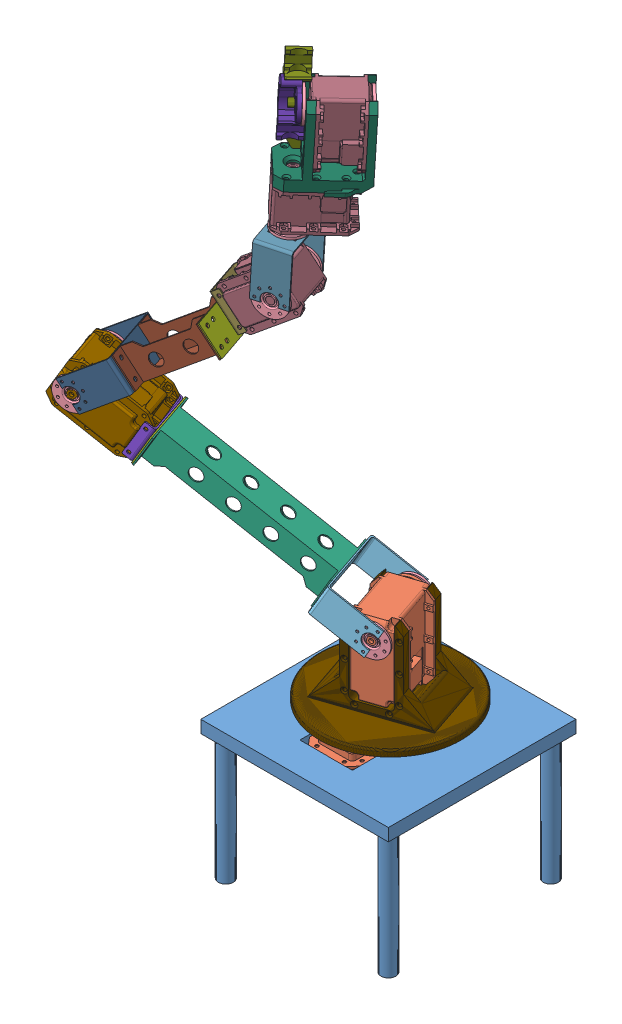
SolidWorks assembly Crust crawler, configuration Default. Lengths in mm.
Overall size (286.73 536.38 160.83).
31 component instances, 18 part files, 69 mates.
Components (placement in the parent):
- Base-1: Base [Default] at (55.1013 113.759 122.0745) size (150 110 150)
- MX-106T-1: MX-106T [Default] at (56.0013 106.759 121.3245) x (1 0 0) z (0 1 0) size (40.2 65.92 55.3)
- Base-disc-1: Base-disc [Default] at (56.0013 136.559 121.3245) x (-0.957483 0 0.288489) z (-0.288489 0 -0.957483) size (110 1 110)
- MX-106T-2: MX-106T [Default] at (55.9531 193.559 121.3159) x (-0.946958 0 0.321357) z (-0.321357 0 -0.946958) size (40.2 65.92 55.3)
- Servo-Disc-2: Servo-Disc [Default] at (46.698 193.559 94.0435) x (-0.321357 0 -0.946958) z (0.946958 0 -0.321357) size (2 25 25)
- Servo-Disc-3: Servo-Disc [Default] at (63.1836 193.559 142.6225) x (0.321357 0 0.946958) z (-0.826712 0.487687 0.28055) size (2 25 25)
- Servo-disc-link_MX-106T-2: Servo-disc-link_MX-106T [Default] at (15.7767 201.1783 125.1291) x (0.321357 0 0.946958) z (-0.826712 0.487687 0.28055) size (57.3 25 41)
- Link-1-1: Link-1 [Default] at (-24.8512 254.9473 145.4109) x (-0.321357 0 -0.946958) z (-0.826712 0.487687 0.28055) size (45 25 130)
- Link-plate-1: Link-plate [Default] at (-84.3602 275.7342 165.6057) x (-0.321357 0 -0.946958) z (-0.826712 0.487687 0.28055) size (45 25 1)
- Servo-link-link_MX-64T-1: Servo-link-link_MX-64T [Default] at (-93.9736 263.3704 164.1161) x (-0.321357 0 -0.946958) z (0.826712 -0.487687 -0.28055) size (36 30 8)
- MX-64T-1: MX-64T [Default] at (-126.7705 300.7525 179.998) x (-0.461819 -0.873019 0.156721) z (-0.321357 0 -0.946958) size (40.2 62.1 50)
- Servo-Disc-4: Servo-Disc [Default] at (-135.1258 300.7525 155.3771) x (-0.321357 0 -0.946958) z (0.934807 -0.159687 -0.317233) size (2 25 25)
- Servo-Disc-5: Servo-Disc [Default] at (-120.3434 300.7525 198.9372) x (0.321357 0 0.946958) z (0.288069 0.952607 -0.097758) size (2 25 25)
- Servo-disc-link_MX-64T-1: Servo-disc-link_MX-64T [Default] at (-90.5023 312.8501 168.2181) x (-0.321357 0 -0.946958) z (0.767934 0.585117 -0.260604) size (52 25 41)
- Link-2-1: Link-2 [Default] at (-65.5173 332.7441 156.0432) x (-0.321357 0 -0.946958) z (0.767934 0.585117 -0.260604) size (45 25 67)
- Link-plate-2: Link-plate [Default] at (-46.7175 362.4824 149.6634) x (0.321357 0 0.946958) z (0.767934 0.585117 -0.260604) size (45 25 1)
- Servo-link-link_MX-28T-1: Servo-link-link_MX-28T [Default] at (-42.8849 355.2506 138.9643) x (0.321357 0 0.946958) z (-0.767934 -0.585117 0.260604) size (32 30 8)
- MX-28T-1: MX-28T [Default] at (-22.3058 390.9491 125.1165) x (0.554082 -0.810949 -0.188031) z (0.321357 0 0.946958) size (35.6 50.71 41.85)
- Servo-Disc-6: Servo-Disc [Default] at (-15.6858 390.9491 144.6239) x (0.321357 0 0.946958) z (0.945652 -0.052502 -0.320914) size (2 25 25)
- Servo-Disc-8: Servo-Disc [Default] at (-27.8492 390.9491 108.7815) x (-0.321357 0 -0.946958) z (0.909105 -0.279908 -0.308511) size (2 25 25)
- Servo-disc-link_MX-28T-2: Servo-disc-link_MX-28T [Default] at (-31.5141 429.553 130.6175) x (0.321357 0 0.946958) z (0.049717 0.998621 -0.016872) size (43.85 25 41)
- Servo-Disc-10: Servo-Disc [Default] at (-19.754 431.3933 126.0194) x (-0.049717 -0.998621 0.016872) z (0.75968 -0.048777 -0.648465) size (2 25 25)
- Servo-Disc-11: Servo-Disc [Default] at (-17.8722 469.1911 125.3808) x (0.049717 0.998621 -0.016872) z (0.847678 -0.033257 0.529468) size (2 25 25)
- MX-28T-3: MX-28T [Default] at (-18.7298 451.9649 125.6718) x (0.730716 -0.024853 0.682229) z (-0.049717 -0.998621 0.016872) size (35.6 50.71 41.85)
- Holder-thing.step-1: Holder-thing.step [Default] at (75.6346 363.141 21.365) x (0.730716 -0.024853 0.682229) z (-0.049717 -0.998621 0.016872) size (39.6 57 61.2)
- Servo-Disc-12: Servo-Disc [Default] at (-12.5421 515.8728 121.3725) x (-0.680869 0.046247 0.730944) z (0.732405 0.043319 0.679489) size (2 25 25)
- Servo-Disc-13: Servo-Disc [Default] at (13.2288 514.1224 93.7063) x (0.680869 -0.046247 -0.730944) z (0.437057 -0.775176 0.456161) size (2 25 25)
- MX-28T-4: MX-28T [Default] at (1.4838 514.9201 106.315) x (0.730716 -0.024853 0.682229) z (-0.680869 0.046247 0.730944) size (35.6 50.71 41.85)
- Gripper1.step-1: Gripper1.step [Default] at (75.9901 361.3633 20.9195) x (0.730716 -0.024853 0.682229) z (-0.049717 -0.998621 0.016872) size (17.31 15.51 73.9)
- Gripper2.step-1: Gripper2.step [Default] at (99.7904 656.3992 27.1583) x (-0.722497 0.121196 -0.680669) z (0.120066 0.991551 0.049105) size (28 15.5 49.84)
- NewBase.step-1: NewBase.step [Default] at (56.1028 137.9928 120.7961) x (0.946832 0 -0.321728) z (0 1 0) size (112.99 113 71)
Mates (geometry in assembly coordinates):
- Coincident3: coincident aligned: plane of Base-1 through (55.1013 123.759 122.0745) normal (0 1 0); plane of MX-106T-1 through (35.0973 123.759 173.2265) normal (0 1 0)
- Concentric1: concentric anti-aligned: cylinder of MX-106T-1 through (56.0013 137.559 121.3245) axis (0 -1 0) radius 2.75; cylinder of Base-disc-1 through (56.0013 136.559 121.3245) axis (0 1 0) radius 3
- Coincident4: coincident aligned: plane of MX-106T-1 through (58.8652 137.559 118.4606) normal (0 1 0); plane of Base-disc-1 through (56.0013 137.559 121.3245) normal (0 1 0)
- Coincident5: coincident: plane of Base-1 through (55.1013 13.759 106.8245) normal (0 0 1); plane of MX-106T-1 through (71.6013 84.899 106.8245) normal (0 0 -1)
- Coincident6: coincident anti-aligned: plane of Base-1 through (76.1013 13.759 122.0745) normal (-1 0 0); plane of MX-106T-1 through (76.1013 120.145 166.9865) normal (1 0 0)
- Parallel1: parallel: plane of Base-1 through (55.1013 123.759 122.0745) normal (0 1 0); plane of MX-106T-1 through (35.0973 123.759 173.2265) normal (0 1 0)
- Concentric4: concentric aligned: circle of MX-106T-2; circle of Servo-Disc-2
- Coincident13: coincident aligned: plane of MX-106T-2 through (43.3433 196.4229 93.0699) normal (-0.321357 0 -0.946958); plane of Servo-Disc-2 through (46.0553 193.559 92.1496) normal (-0.321357 0 -0.946958)
- Concentric5: concentric aligned: circle of MX-106T-2; circle of Servo-Disc-3
- Coincident14: coincident: plane of MX-106T-2 through (59.8788 197.719 145.856) normal (0.321357 0 0.946958); plane of Servo-Disc-3 through (63.8263 193.559 144.5164) normal (0.321357 0 0.946958)
- Coincident15: coincident aligned: circle of Servo-Disc-3; circle of Servo-disc-link_MX-106T-2
- Coincident16: coincident: circle of Servo-Disc-3; circle of Servo-disc-link_MX-106T-2
- Coincident18: coincident aligned: circle of Servo-disc-link_MX-106T-2; circle of Link-1-1
- Coincident22: coincident aligned: circle of Servo-disc-link_MX-106T-2; circle of Link-1-1
- Coincident23: coincident: circle of Link-1-1; circle of Link-plate-1
- Coincident24: coincident aligned: circle of Link-1-1; circle of Link-plate-1
- Coincident27: coincident anti-aligned: circle of Link-plate-1; circle of Servo-link-link_MX-64T-1
- Coincident32: coincident anti-aligned: circle of Link-plate-1; circle of Servo-link-link_MX-64T-1
- Coincident33: coincident anti-aligned: circle of Servo-link-link_MX-64T-1; circle of MX-64T-1
- Coincident34: coincident anti-aligned: circle of Servo-link-link_MX-64T-1; circle of MX-64T-1
- Concentric6: concentric aligned: cylinder of MX-64T-1 through (-135.7685 300.7525 153.4832) axis (0.321357 0 0.946958) radius 2.75; cylinder of Servo-Disc-4 through (-135.7685 300.7525 153.4832) axis (0.321357 0 0.946958) radius 3
- Coincident35: coincident aligned: plane of MX-64T-1 through (-139.4563 299.6456 154.7346) normal (-0.321357 0 -0.946958); plane of Servo-Disc-4 through (-135.7685 300.7525 153.4832) normal (-0.321357 0 -0.946958)
- Concentric7: concentric anti-aligned: circle of MX-64T-1; cylinder of Servo-Disc-5 through (-119.7007 300.7525 200.8311) axis (-0.321357 0 -0.946958) radius 3
- Coincident36: coincident aligned: plane of MX-64T-1 through (-125.061 299.1495 202.6501) normal (0.321357 0 0.946958); plane of Servo-Disc-5 through (-119.7007 300.7525 200.8311) normal (0.321357 0 0.946958)
- Coincident37: coincident aligned: circle of Servo-Disc-4; circle of Servo-disc-link_MX-64T-1
- Coincident38: coincident aligned: circle of Servo-Disc-4; circle of Servo-disc-link_MX-64T-1
- Coincident39: coincident aligned: circle of Servo-disc-link_MX-64T-1; circle of Link-2-1
- Coincident40: coincident aligned: circle of Servo-disc-link_MX-64T-1; circle of Link-2-1
- Concentric9: concentric anti-aligned: cylinder of MX-28T-1 through (-16.6017 390.9491 141.925) axis (0.321357 0 0.946958) radius 2.85; cylinder of Servo-Disc-6 through (-15.0431 390.9491 146.5178) axis (-0.321357 0 -0.946958) radius 3
- Coincident61: coincident aligned: plane of MX-28T-1 through (-18.9663 391.6149 147.8491) normal (0.321357 0 0.946958); plane of Servo-Disc-6 through (-15.0431 390.9491 146.5178) normal (0.321357 0 0.946958)
- Coincident63: coincident aligned: plane of MX-28T-1 through (-24.3636 390.2393 105.4866) normal (-0.321357 0 -0.946958); plane of Servo-Disc-8 through (-28.4919 390.9491 106.8876) normal (-0.321357 0 -0.946958)
- Concentric11: concentric anti-aligned: cylinder of MX-28T-1 through (-27.7849 390.9491 108.9709) axis (-0.321357 0 -0.946958) radius 3; cylinder of Servo-Disc-8 through (-28.4919 390.9491 106.8876) axis (0.321357 0 0.946958) radius 3
- Coincident66: coincident aligned: circle of Servo-Disc-6; circle of Servo-disc-link_MX-28T-2
- Coincident67: coincident aligned: circle of Servo-Disc-6; circle of Servo-disc-link_MX-28T-2
- Lock1: lock: unknown of Servo-link-link_MX-28T-1; unknown of MX-28T-1
- Parallel24: parallel anti-aligned: line of Link-plate-2 through (-45.091 372.3934 172.8717) axis (0.554082 -0.810949 -0.188031); line of Servo-link-link_MX-28T-1 through (-40.8586 354.958 146.1967) axis (-0.554082 0.810949 0.188031)
- Distance17: distance = 0 mm anti-aligned: plane of Link-plate-2 through (-45.9496 363.0675 149.4028) normal (0.767934 0.585117 -0.260604); plane of Servo-link-link_MX-28T-1 through (-67.1218 379.2865 123.4289) normal (-0.767934 -0.585117 0.260604)
- Parallel27: parallel aligned: line of Link-plate-2 through (-59.7848 373.2043 131.3936) axis (0.321357 0 0.946958); line of Servo-link-link_MX-28T-1 through (-66.4791 379.2865 125.3229) axis (0.321357 0 0.946958)
- Distance19: distance = 2.5 mm: line of Servo-link-link_MX-28T-1 through (-49.8566 354.958 119.6819) axis (0.321357 0 0.946958); line of Link-plate-2 through (-32.1144 352.9306 167.412) axis (-0.321357 0 -0.946958)
- Distance20: distance = 6.9 mm: line of Servo-link-link_MX-28T-1 through (-66.4791 379.2865 125.3229) axis (0.554082 -0.810949 -0.188031); line of Link-plate-2 through (-46.8082 353.7416 125.9339) axis (-0.554082 0.810949 0.188031)
- Coincident115: coincident aligned: circle of Link-2-1; circle of Link-plate-2
- Coincident116: coincident aligned: circle of Link-2-1; circle of Link-plate-2
- Coincident117: coincident aligned: plane of Servo-Disc-10 through (-19.8534 429.396 126.0531) normal (-0.049717 -0.998621 0.016872); plane of MX-28T-3 through (-19.9969 429.3323 121.86) normal (-0.049717 -0.998621 0.016872)
- Concentric14: concentric anti-aligned: cylinder of Servo-Disc-11 through (-17.7727 471.1883 125.347) axis (-0.049717 -0.998621 0.016872) radius 3; cylinder of MX-28T-3 through (-17.8821 468.9914 125.3841) axis (0.049717 0.998621 -0.016872) radius 3
- Concentric15: concentric anti-aligned: cylinder of Servo-Disc-10 through (-19.8534 429.396 126.0531) axis (0.049717 0.998621 -0.016872) radius 3; cylinder of MX-28T-3 through (-19.6123 434.2393 125.9713) axis (-0.049717 -0.998621 0.016872) radius 2.85
- Coincident118: coincident aligned: plane of Servo-Disc-11 through (-17.7727 471.1883 125.347) normal (0.049717 0.998621 -0.016872); plane of MX-28T-3 through (-17.6125 471.2549 129.7606) normal (0.049717 0.998621 -0.016872)
- ProfileCenter1: profile center = 0 mm anti-aligned: plane of Servo-disc-link_MX-28T-2 through (-15.0785 428.7398 101.2796) normal (0.049717 0.998621 -0.016872); circle of Servo-Disc-10
- Coincident123: coincident anti-aligned: plane of MX-28T-3 through (-4.5405 465.5723 83.8352) normal (0.049717 0.998621 -0.016872); plane of Holder-thing.step-1 through (-8.9285 466.3291 115.6972) normal (-0.049717 -0.998621 0.016872)
- Concentric17: concentric aligned: cylinder of MX-28T-3 through (0.0557 463.0032 93.4942) axis (0.049717 0.998621 -0.016872) radius 1.35; cylinder of Holder-thing.step-1 through (0.4286 470.4929 93.3676) axis (0.049717 0.998621 -0.016872) radius 1.35
- Concentric18: concentric aligned: cylinder of MX-28T-3 through (-32.133 465.0285 118.5167) axis (0.049717 0.998621 -0.016872) radius 1.35; cylinder of Holder-thing.step-1 through (-31.7601 472.5182 118.3902) axis (0.049717 0.998621 -0.016872) radius 1.35
- Coincident124: coincident aligned: plane of Servo-Disc-12 through (-13.9038 515.9653 122.8344) normal (-0.680869 0.046247 0.730944); plane of MX-28T-4 through (-16.2174 513.0729 120.8623) normal (-0.680869 0.046247 0.730944)
- Concentric19: concentric anti-aligned: cylinder of Servo-Disc-13 through (14.5905 514.0299 92.2444) axis (-0.680869 0.046247 0.730944) radius 3; cylinder of MX-28T-4 through (13.0926 514.1316 93.8524) axis (0.680869 -0.046247 -0.730944) radius 3
- Concentric20: concentric anti-aligned: cylinder of Servo-Disc-12 through (-13.9038 515.9653 122.8344) axis (0.680869 -0.046247 -0.730944) radius 3; cylinder of MX-28T-4 through (-10.6016 515.741 119.2893) axis (-0.680869 0.046247 0.730944) radius 2.85
- Coincident125: coincident aligned: plane of Servo-Disc-13 through (14.5905 514.0299 92.2444) normal (0.680869 -0.046247 -0.730944); plane of MX-28T-4 through (17.0302 517.0679 94.3247) normal (0.680869 -0.046247 -0.730944)
- Coincident126: coincident anti-aligned: plane of Holder-thing.step-1 through (-10.4246 481.5609 117.8545) normal (0.680869 -0.046247 -0.730944); plane of MX-28T-4 through (-24.2257 476.5166 105.3181) normal (-0.680869 0.046247 0.730944)
- Concentric22: concentric anti-aligned: cylinder of Holder-thing.step-1 through (-4.298 479.652 123.6822) axis (-0.680869 0.046247 0.730944) radius 1.35; cylinder of MX-28T-4 through (-4.298 479.652 123.6822) axis (0.680869 -0.046247 -0.730944) radius 1.35
- Concentric23: concentric anti-aligned: cylinder of Holder-thing.step-1 through (-0.7424 519.2086 86.8689) axis (-0.680869 0.046247 0.730944) radius 1.35; cylinder of MX-28T-4 through (-19.4663 520.4804 106.9698) axis (0.680869 -0.046247 -0.730944) radius 1.35
- Coincident127: coincident anti-aligned: plane of Holder-thing.step-1 through (-14.2375 481.8199 121.9478) normal (-0.680869 0.046247 0.730944); plane of Gripper1.step-1 through (-20.9092 535.1529 112.3587) normal (0.680869 -0.046247 -0.730944)
- Coincident128: coincident anti-aligned: circle of Holder-thing.step-1; circle of Gripper1.step-1
- Coincident129: coincident anti-aligned: circle of Holder-thing.step-1; circle of Gripper1.step-1
- Coincident130: coincident anti-aligned: plane of Base-disc-1 through (56.0013 137.559 121.3245) normal (0 1 0); plane of NewBase.step-1 through (11.9556 137.559 156.7626) normal (0 -1 0)
- Coincident132: coincident anti-aligned: plane of MX-106T-2 through (70.2853 141.657 98.5) normal (-0.321357 0 -0.946958); plane of NewBase.step-1 through (35.087 174.6912 110.4448) normal (0.321357 0 0.946958)
- Concentric29: concentric aligned: circle of Base-disc-1; circle of NewBase.step-1
- Coincident139: coincident: point of MX-106T-2; point of NewBase.step-1
- Coincident140: coincident: circle of MX-106T-2; point of NewBase.step-1
- Coincident142: coincident: circle of MX-106T-2; point of NewBase.step-1
- Coincident143: coincident: circle of MX-106T-2; point of NewBase.step-1
- Tangent5: tangent: circle of Servo-Disc-12; circle of Gripper2.step-1
- Concentric31: concentric anti-aligned: circle of Servo-Disc-12; circle of Gripper2.step-1
